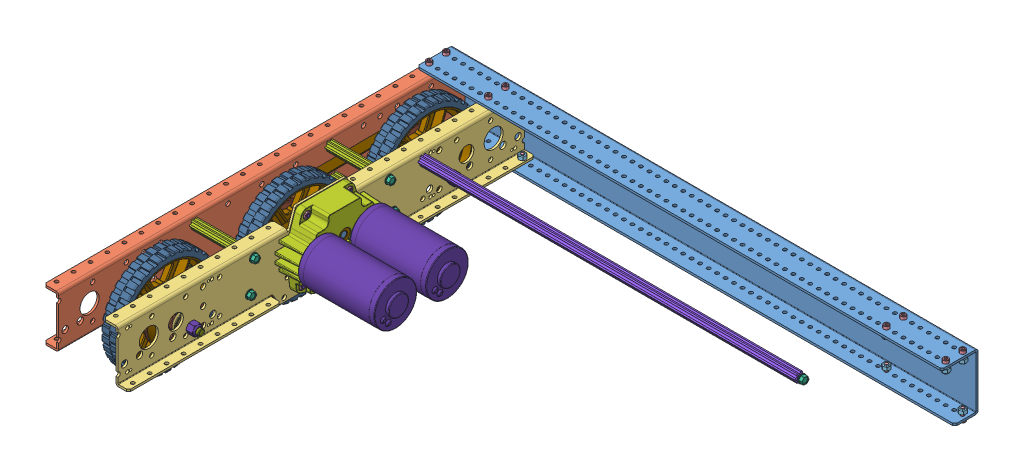
SolidWorks assembly AM14U4 Wide Half, configuration Default. Lengths in mm.
Overall size (788.5 213.52 613.54).
149 component instances, 36 part files, 33 mates.
Components (placement in the parent):
- AM14U4 Wide Frame Half-1: AM14U4 Wide Frame Half [Default] at (335.1417 50.6739 -281.2356) size (788.5 116.33 613.54)
  - am-xxxx AM14U4 End Plate-1: am-xxxx AM14U4 End Plate [Default] at (-787.4 -81.407 -3.175) x (1 0 0) z (0 -1 0) size (787.4 53.98 84.58)
  - am-xxxx AM14U4 Outside Plate Wide-1: am-xxxx AM14U4 Outside Plate Wide [DefaultSM-FLAT-PATTERN] at (-768.35 -77.216 711.962) x (0 0 -1) z (0 -1 0) size (609.6 22.23 77.72)
  - am-xxxx AM14U4 Inside Plate Wide-1: am-xxxx AM14U4 Inside Plate Wide [Default] at (-679.45 -77.216 711.962) x (0 0 -1) z (0 -1 0) size (609.6 38.1 116.33)
  - am-1002 and am-1042 10-32 x 0500 and Nylock Nut Assembly-1: am-1002 and am-1042 10-32 x 0500 and Nylock Nut Assembly [Default] at (-784.5821 -6.6363 35.2132) x (0 -1 0) z (0 0 1) size (17.53 13.8 13)
    - 10-32x0500_shcs-1: 10-32x0500_shcs [HX-SHCS 0.19-32x1.375x1-C] at (-11.4623 3.5321 3.6488) size (17.53 7.94 7.94)
    - 10-32 Nylock Nut 1-1: 10-32 Nylock Nut 1 [90631A411] at (-0.0323 3.5321 3.6488) x (0 0.381849 -0.924225) z (0 -0.924225 -0.381849) size (9.53 6.11 11)
  - am-1002 and am-1042 10-32 x 0500 and Nylock Nut Assembly-2: am-1002 and am-1042 10-32 x 0500 and Nylock Nut Assembly [Default] at (-784.5821 -6.6363 9.8132) x (0 -1 0) z (0 0 1) size (17.53 13.8 13)
    - 10-32x0500_shcs-1: 10-32x0500_shcs [HX-SHCS 0.19-32x1.375x1-C] at (-11.4623 3.5321 3.6488) size (17.53 7.94 7.94)
    - 10-32 Nylock Nut 1-1: 10-32 Nylock Nut 1 [90631A411] at (-0.0323 3.5321 3.6488) x (0 0.381849 -0.924225) z (0 -0.924225 -0.381849) size (9.53 6.11 11)
  - am-1002 and am-1042 10-32 x 0500 and Nylock Nut Assembly-3: am-1002 and am-1042 10-32 x 0500 and Nylock Nut Assembly [Default] at (-695.6821 -6.6363 35.2132) x (0 -1 0) z (0 0 1) size (17.53 13.8 13)
    - 10-32x0500_shcs-1: 10-32x0500_shcs [HX-SHCS 0.19-32x1.375x1-C] at (-11.4623 3.5321 3.6488) size (17.53 7.94 7.94)
    - 10-32 Nylock Nut 1-1: 10-32 Nylock Nut 1 [90631A411] at (-0.0323 3.5321 3.6488) x (0 0.381849 -0.924225) z (0 -0.924225 -0.381849) size (9.53 6.11 11)
  - am-1002 and am-1042 10-32 x 0500 and Nylock Nut Assembly-4: am-1002 and am-1042 10-32 x 0500 and Nylock Nut Assembly [Default] at (-695.6821 -6.6363 9.8132) x (0 -1 0) z (0 0 1) size (17.53 13.8 13)
    - 10-32x0500_shcs-1: 10-32x0500_shcs [HX-SHCS 0.19-32x1.375x1-C] at (-11.4623 3.5321 3.6488) size (17.53 7.94 7.94)
    - 10-32 Nylock Nut 1-1: 10-32 Nylock Nut 1 [90631A411] at (-0.0323 3.5321 3.6488) x (0 0.381849 -0.924225) z (0 -0.924225 -0.381849) size (9.53 6.11 11)
  - am-1002 and am-1042 10-32 x 0500 and Nylock Nut Assembly-5: am-1002 and am-1042 10-32 x 0500 and Nylock Nut Assembly [Default] at (-777.5179 -77.9457 9.8132) x (0 1 0) z (0 0 1) size (17.53 13.8 13)
    - 10-32x0500_shcs-1: 10-32x0500_shcs [HX-SHCS 0.19-32x1.375x1-C] at (-11.4623 3.5321 3.6488) size (17.53 7.94 7.94)
    - 10-32 Nylock Nut 1-1: 10-32 Nylock Nut 1 [90631A411] at (-0.0323 3.5321 3.6488) x (0 0.381849 -0.924225) z (0 -0.924225 -0.381849) size (9.53 6.11 11)
  - am-1002 and am-1042 10-32 x 0500 and Nylock Nut Assembly-6: am-1002 and am-1042 10-32 x 0500 and Nylock Nut Assembly [Default] at (-663.2179 -77.9457 9.8132) x (0 1 0) z (0 0 1) size (17.53 13.8 13)
    - 10-32x0500_shcs-1: 10-32x0500_shcs [HX-SHCS 0.19-32x1.375x1-C] at (-11.4623 3.5321 3.6488) size (17.53 7.94 7.94)
    - 10-32 Nylock Nut 1-1: 10-32 Nylock Nut 1 [90631A411] at (-0.0323 3.5321 3.6488) x (0 0.381849 -0.924225) z (0 -0.924225 -0.381849) size (9.53 6.11 11)
  - am-1002 and am-1042 10-32 x 0500 and Nylock Nut Assembly-7: am-1002 and am-1042 10-32 x 0500 and Nylock Nut Assembly [Default] at (-2.8179 -77.9457 9.8132) x (0 1 0) z (0 0 1) size (17.53 13.8 13)
    - 10-32x0500_shcs-1: 10-32x0500_shcs [HX-SHCS 0.19-32x1.375x1-C] at (-11.4623 3.5321 3.6488) size (17.53 7.94 7.94)
    - 10-32 Nylock Nut 1-1: 10-32 Nylock Nut 1 [90631A411] at (-0.0323 3.5321 3.6488) x (0 0.381849 -0.924225) z (0 -0.924225 -0.381849) size (9.53 6.11 11)
  - am-1002 and am-1042 10-32 x 0500 and Nylock Nut Assembly-8: am-1002 and am-1042 10-32 x 0500 and Nylock Nut Assembly [Default] at (-9.8821 -6.6363 9.8132) x (0 -1 0) z (0 0 1) size (17.53 13.8 13)
    - 10-32x0500_shcs-1: 10-32x0500_shcs [HX-SHCS 0.19-32x1.375x1-C] at (-11.4623 3.5321 3.6488) size (17.53 7.94 7.94)
    - 10-32 Nylock Nut 1-1: 10-32 Nylock Nut 1 [90631A411] at (-0.0323 3.5321 3.6488) x (0 0.381849 -0.924225) z (0 -0.924225 -0.381849) size (9.53 6.11 11)
  - am-1002 and am-1042 10-32 x 0500 and Nylock Nut Assembly-9: am-1002 and am-1042 10-32 x 0500 and Nylock Nut Assembly [Default] at (-9.8821 -6.6363 35.2132) x (0 -1 0) z (0 0 1) size (17.53 13.8 13)
    - 10-32x0500_shcs-1: 10-32x0500_shcs [HX-SHCS 0.19-32x1.375x1-C] at (-11.4623 3.5321 3.6488) size (17.53 7.94 7.94)
    - 10-32 Nylock Nut 1-1: 10-32 Nylock Nut 1 [90631A411] at (-0.0323 3.5321 3.6488) x (0 0.381849 -0.924225) z (0 -0.924225 -0.381849) size (9.53 6.11 11)
  - am-1002 and am-1042 10-32 x 0500 and Nylock Nut Assembly-10: am-1002 and am-1042 10-32 x 0500 and Nylock Nut Assembly [Default] at (-98.7821 -6.6363 9.8132) x (0 -1 0) z (0 0 1) size (17.53 13.8 13)
    - 10-32x0500_shcs-1: 10-32x0500_shcs [HX-SHCS 0.19-32x1.375x1-C] at (-11.4623 3.5321 3.6488) size (17.53 7.94 7.94)
    - 10-32 Nylock Nut 1-1: 10-32 Nylock Nut 1 [90631A411] at (-0.0323 3.5321 3.6488) x (0 0.381849 -0.924225) z (0 -0.924225 -0.381849) size (9.53 6.11 11)
  - am-1002 and am-1042 10-32 x 0500 and Nylock Nut Assembly-11: am-1002 and am-1042 10-32 x 0500 and Nylock Nut Assembly [Default] at (-98.7821 -6.6363 35.2132) x (0 -1 0) z (0 0 1) size (17.53 13.8 13)
    - 10-32x0500_shcs-1: 10-32x0500_shcs [HX-SHCS 0.19-32x1.375x1-C] at (-11.4623 3.5321 3.6488) size (17.53 7.94 7.94)
    - 10-32 Nylock Nut 1-1: 10-32 Nylock Nut 1 [90631A411] at (-0.0323 3.5321 3.6488) x (0 0.381849 -0.924225) z (0 -0.924225 -0.381849) size (9.53 6.11 11)
  - am-1002 and am-1042 10-32 x 0500 and Nylock Nut Assembly-12: am-1002 and am-1042 10-32 x 0500 and Nylock Nut Assembly [Default] at (-117.1179 -77.9457 9.8132) x (0 1 0) z (0 0 1) size (17.53 13.8 13)
    - 10-32x0500_shcs-1: 10-32x0500_shcs [HX-SHCS 0.19-32x1.375x1-C] at (-11.4623 3.5321 3.6488) size (17.53 7.94 7.94)
    - 10-32 Nylock Nut 1-1: 10-32 Nylock Nut 1 [90631A411] at (-0.0323 3.5321 3.6488) x (0 0.381849 -0.924225) z (0 -0.924225 -0.381849) size (9.53 6.11 11)
  - FHTS 0.25-20-0.75-1: FHTS 0.25-20-0.75 [FHTS 0.25-20-G-0.75-C] at (-768.35 -59.6687 198.0365) size (24.64 12.19 12.19)
  - FHTS 0.25-20-0.75-2: FHTS 0.25-20-0.75 [FHTS 0.25-20-G-0.75-C] at (-768.35 -14.986 203.962) size (24.64 12.19 12.19)
  - FHTS 0.25-20-0.75-3: FHTS 0.25-20-0.75 [FHTS 0.25-20-G-0.75-C] at (-768.35 -14.986 407.162) size (24.64 12.19 12.19)
  - FHTS 0.25-20-0.75-4: FHTS 0.25-20-0.75 [FHTS 0.25-20-G-0.75-C] at (-768.35 -59.6687 413.0875) size (24.64 12.19 12.19)
  - FHTS 0.25-20-0.75-5: FHTS 0.25-20-0.75 [FHTS 0.25-20-G-0.75-C] at (-676.275 -59.6687 413.0875) x (-1 0 0) z (0 0.924225 0.381849) size (24.64 12.19 12.19)
  - FHTS 0.25-20-0.75-6: FHTS 0.25-20-0.75 [FHTS 0.25-20-G-0.75-C] at (-676.275 -14.986 407.162) x (-1 0 0) z (0 0.924225 0.381849) size (24.64 12.19 12.19)
  - FHTS 0.25-20-0.75-7: FHTS 0.25-20-0.75 [FHTS 0.25-20-G-0.75-C] at (-676.275 -14.986 203.962) x (-1 0 0) z (0 0.924225 0.381849) size (24.64 12.19 12.19)
  - FHTS 0.25-20-0.75-8: FHTS 0.25-20-0.75 [FHTS 0.25-20-G-0.75-C] at (-676.275 -59.6687 198.0365) x (-1 0 0) z (0 0.924225 0.381849) size (24.64 12.19 12.19)
  - 3.375in Churro-1: 3.375in Churro [Default] at (-679.45 -59.6687 198.0365) x (0 0 1) z (-1 0 0) size (14.66 12.7 85.72)
  - 3.375in Churro-2: 3.375in Churro [Default] at (-679.45 -14.986 203.962) x (0 0 1) z (-1 0 0) size (14.66 12.7 85.72)
  - 3.375in Churro-3: 3.375in Churro [Default] at (-679.45 -14.986 407.162) x (0 0 1) z (-1 0 0) size (14.66 12.7 85.72)
  - 3.375in Churro-4: 3.375in Churro [Default] at (-679.45 -59.6687 413.0875) x (0 0 1) z (-1 0 0) size (14.66 12.7 85.72)
  - 22.25in Churro-1: 22.25in Churro [Default] at (-393.7 -14.986 153.162) x (0 0 -1) z (1 0 0) size (14.66 12.7 565.15)
  - FHTS 0.25-20-0.75-9: FHTS 0.25-20-0.75 [FHTS 0.25-20-G-0.75-C] at (-107.95 -14.986 153.162) x (-1 0 0) z (0 0.924225 0.381849) size (24.64 12.19 12.19)
- 6 HiGrip with bearings, pulleys and spacers-1: 6 HiGrip with bearings, pulleys and spacers [Default] at (-418.7948 -84.3541 86.993) size (85.56 152.4 152.4)
  - 6 HiGrip Asm Rev II-1: 6 HiGrip Asm Rev II [Default] at (83.7987 67.439 110.9939) size (35.05 152.4 152.4)
    - 6 wheel Rev 4-1: 6 wheel Rev 4 [Default] at (-52.6446 9.4231 21.378) size (35.05 132.08 132.08)
    - 6 wheel tread II-1: 6 wheel tread II [Default] at (-65.3446 9.4231 21.378) x (0 0 -1) z (1 0 0) size (152.4 152.4 25.58)
  - 42 tooth HTD Pulley half 2014-1: 42 tooth HTD Pulley half 2014 [Default] at (47.6006 76.862 132.3719) x (1 0 0) z (0 -0.5 0.866025) size (13 74.23 74.23)
  - 42 tooth HTD Pulley half 2014-2: 42 tooth HTD Pulley half 2014 [Default] at (64.263 76.862 132.3719) x (-1 0 0) z (0 -0.499927 0.866067) size (13 74.23 74.23)
  - 1614Z Bearing-1: 1614Z Bearing [Default] at (62.612 76.862 132.3719) x (0 -0.157148 -0.987575) z (-1 0 0) size (28.57 28.57 9.53)
  - 10-24 Hex Washer Rolling x 1.25-1: 10-24 Hex Washer Rolling x 1.25 [93882A213] at (63.247 76.8605 108.5602) x (0 0 -1) z (1 0 0) size (10.52 10.52 35.59)
  - 10-24 Hex Washer Rolling x 1.25-2: 10-24 Hex Washer Rolling x 1.25 [93882A213] at (63.247 97.4833 120.4656) x (0 0 -1) z (1 0 0) size (10.52 10.52 35.59)
  - 10-24 Hex Washer Rolling x 1.25-3: 10-24 Hex Washer Rolling x 1.25 [93882A213] at (63.247 56.2398 144.2799) x (0 0 -1) z (1 0 0) size (10.52 10.52 35.59)
  - 10-24 Hex Washer Rolling x 1.25-4: 10-24 Hex Washer Rolling x 1.25 [93882A213] at (63.247 76.8625 156.1852) x (0 -0.95788 -0.287168) z (1 0 0) size (10.52 10.52 35.59)
  - 10-24 Hex Washer Rolling x 1.25-5: 10-24 Hex Washer Rolling x 1.25 [93882A213] at (63.247 97.4843 144.2781) x (0 -0.868976 0.494854) z (1 0 0) size (10.52 10.52 35.59)
  - 10-24 Hex Washer Rolling x 1.25-6: 10-24 Hex Washer Rolling x 1.25 [93882A213] at (63.247 56.2388 120.4674) x (0 -0.977348 -0.211637) z (1 0 0) size (10.52 10.52 35.59)
  - am-1306 spacer 0280 WashersUSA 13RS052001-1: am-1306 spacer 0280 WashersUSA 13RS052001 [Default] at (74.4865 76.862 132.3719) x (0 -0.35357 0.935408) z (-1 0 0) size (13.16 13.16 7.11)
  - 1614Z Bearing-2: 1614Z Bearing [Default] at (15.2791 76.862 132.3719) x (0 0.155433 -0.987846) z (-1 0 0) size (28.57 28.57 9.53)
  - am-1307 850 long 380 id-1: am-1307 850 long 380 id [Default] at (10.5166 76.862 132.3719) x (0 0.971418 -0.237374) z (0 0.237374 0.971418) size (19.05 21.59 19.05)
- 6 HiGrip with bearings, pulleys and spacers-2: 6 HiGrip with bearings, pulleys and spacers [Default] at (-355.3817 51.5414 -29.4849) x (-1 0 0) z (0 -0.796812 -0.604227) size (85.56 152.4 152.4)
  - 6 HiGrip Asm Rev II-1: 6 HiGrip Asm Rev II [Default] at (83.7987 67.439 110.9939) size (35.05 152.4 152.4)
    - 6 wheel Rev 4-1: 6 wheel Rev 4 [Default] at (-52.6446 9.4231 21.378) size (35.05 132.08 132.08)
    - 6 wheel tread II-1: 6 wheel tread II [Default] at (-65.3446 9.4231 21.378) x (0 0 -1) z (1 0 0) size (152.4 152.4 25.58)
  - 42 tooth HTD Pulley half 2014-1: 42 tooth HTD Pulley half 2014 [Default] at (47.6006 76.862 132.3719) x (1 0 0) z (0 -0.5 0.866025) size (13 74.23 74.23)
  - 42 tooth HTD Pulley half 2014-2: 42 tooth HTD Pulley half 2014 [Default] at (64.263 76.862 132.3719) x (-1 0 0) z (0 -0.499927 0.866067) size (13 74.23 74.23)
  - 1614Z Bearing-1: 1614Z Bearing [Default] at (62.612 76.862 132.3719) x (0 -0.157148 -0.987575) z (-1 0 0) size (28.57 28.57 9.53)
  - 10-24 Hex Washer Rolling x 1.25-1: 10-24 Hex Washer Rolling x 1.25 [93882A213] at (63.247 76.8605 108.5602) x (0 0 -1) z (1 0 0) size (10.52 10.52 35.59)
  - 10-24 Hex Washer Rolling x 1.25-2: 10-24 Hex Washer Rolling x 1.25 [93882A213] at (63.247 97.4833 120.4656) x (0 0 -1) z (1 0 0) size (10.52 10.52 35.59)
  - 10-24 Hex Washer Rolling x 1.25-3: 10-24 Hex Washer Rolling x 1.25 [93882A213] at (63.247 56.2398 144.2799) x (0 0 -1) z (1 0 0) size (10.52 10.52 35.59)
  - 10-24 Hex Washer Rolling x 1.25-4: 10-24 Hex Washer Rolling x 1.25 [93882A213] at (63.247 76.8625 156.1852) x (0 -0.95788 -0.287168) z (1 0 0) size (10.52 10.52 35.59)
  - 10-24 Hex Washer Rolling x 1.25-5: 10-24 Hex Washer Rolling x 1.25 [93882A213] at (63.247 97.4843 144.2781) x (0 -0.868976 0.494854) z (1 0 0) size (10.52 10.52 35.59)
  - 10-24 Hex Washer Rolling x 1.25-6: 10-24 Hex Washer Rolling x 1.25 [93882A213] at (63.247 56.2388 120.4674) x (0 -0.977348 -0.211637) z (1 0 0) size (10.52 10.52 35.59)
  - am-1306 spacer 0280 WashersUSA 13RS052001-1: am-1306 spacer 0280 WashersUSA 13RS052001 [Default] at (74.4865 76.862 132.3719) x (0 -0.35357 0.935408) z (-1 0 0) size (13.16 13.16 7.11)
  - 1614Z Bearing-2: 1614Z Bearing [Default] at (15.2791 76.862 132.3719) x (0 0.155433 -0.987846) z (-1 0 0) size (28.57 28.57 9.53)
  - am-1307 850 long 380 id-1: am-1307 850 long 380 id [Default] at (10.5166 76.862 132.3719) x (0 0.971418 -0.237374) z (0 0.237374 0.971418) size (19.05 21.59 19.05)
- 375-16 x 4.25 Hex Bolt-1: 375-16 x 4.25 Hex Bolt [HFBOLT 0.375-16x2.5x1-C] at (-439.3805 -7.4921 -170.7121) size (114.12 16.48 14.27)
- 375-16 x 4.25 Hex Bolt-2: 375-16 x 4.25 Hex Bolt [HFBOLT 0.375-16x2.5x1-C] at (-439.3805 -7.4921 219.3649) size (114.12 16.48 14.27)
- 3-8-16 NyLock Nut - Mcm 95615A140-1: 3-8-16 NyLock Nut - Mcm 95615A140 [95615A140] at (-341.1333 -7.4921 -170.7121) x (0 -1 0) z (0 0 1) size (14.29 12 16.5)
- 3-8-16 NyLock Nut - Mcm 95615A140-2: 3-8-16 NyLock Nut - Mcm 95615A140 [95615A140] at (-341.1333 -7.4921 219.3649) x (0 -1 0) z (0 0 1) size (14.29 12 16.5)
- FR8ZZ Hex Bearing-1: FR8ZZ Hex Bearing [Default] at (-436.4366 -9.2701 24.3264) x (0 0 -1) z (1 0 0) size (31.12 31.12 7.93)
- am-2598_107 2016 KOP Toughbox Mini-1: am-2598_107 2016 KOP Toughbox Mini [Default] at (-391.675 -19.3401 115.4272) x (0 0.001296 0.999999) z (-1 0 0) size (140.05 121.81 142.29)
  - Toughbox d07-1: Toughbox d07 [Default] at (-88.5589 93.4503 -52.3959) x (-0.336928 0.94153 0) z (0.94153 0.336928 0) size (11 38.23 9.52)
  - Toughbox d05-1: Toughbox d05 [Default] at (-91.0349 50.9043 -67.5597) x (-0.336928 0.94153 0) z (0 0 -1) size (65.97 66.04 10.16)
  - FR6ZZ Bearing-1: FR6ZZ Bearing [Default] at (-96.247 60.278 -52.5991) x (-0.893862 0.448342 0) z (0 0 1) size (24.69 24.69 7.16)
  - 10-32 Nylock Nut-1: 10-32 Nylock Nut [Default] at (-129.8464 -8.0737 -56.3837) x (0.501678 0.865055 0) z (0 0 -1) size (10.18 11.01 7.1)
  - 10-32 Nylock Nut-2: 10-32 Nylock Nut [Default] at (-59.2462 80.7349 -56.3837) x (0.999999 -0.001296 0) z (0 0 -1) size (10.18 11.01 7.1)
  - 10-32 Nylock Nut-3: 10-32 Nylock Nut [Default] at (-122.7461 80.8172 -56.3837) x (0.500567 0.865698 0) z (0 0 -1) size (10.18 11.01 7.1)
  - 10-32 Nylock Nut-4: 10-32 Nylock Nut [Default] at (-52.3764 -8.1741 -56.3837) x (-0.501678 -0.865055 0) z (0 0 -1) size (10.18 11.01 7.1)
  - 5-16 washer-1: 5-16 washer [Default] at (-52.3162 38.3079 -77.7705) x (0.38418 -0.923258 0) z (0 0 -1) size (17.53 17.53 1.47)
  - 5-16 washer-2: 5-16 washer [Default] at (-52.3162 38.3079 -76.2973) x (0.897267 -0.441488 0) z (0 0 -1) size (17.53 17.53 1.47)
  - 5-16 washer-3: 5-16 washer [Default] at (-129.7861 38.4083 -77.7705) x (-0.990116 0.140253 0) z (0 0 1) size (17.53 17.53 1.47)
  - 5-16 washer-4: 5-16 washer [Default] at (-129.7861 38.4083 -79.2437) x (-0.681761 0.731575 0) z (0 0 1) size (17.53 17.53 1.47)
  - Toughbox d09-1: Toughbox d09 [Default] at (-52.3162 38.3079 -63.5973) x (0.910249 -0.414061 0) z (0 0 -1) size (20.03 20.32 12.7)
  - Toughbox d09-2: Toughbox d09 [Default] at (-129.7861 38.4083 -63.5973) x (0.075368 -0.997156 0) z (0 0 -1) size (20.03 20.32 12.7)
  - TM Housing-1: TM Housing [Default] at (-91.0876 10.1882 -86.3557) x (0.999999 -0.001296 0) z (0 0 1) size (139.9 118.55 41.54)
  - SHCS 10-32 x 0.625-1: SHCS 10-32 x 0.625 [Default] at (-52.2832 63.7078 -74.4685) x (-0.564778 -0.825243 0) z (-0.825243 0.564778 0) size (7.82 20.65 7.82)
  - SHCS 10-32 x 0.625-2: SHCS 10-32 x 0.625 [Default] at (-122.7461 80.8172 -42.5915) x (0.507484 -0.861661 0) z (-0.861661 -0.507484 0) size (7.82 20.65 7.82)
  - SHCS 10-32 x 0.625-3: SHCS 10-32 x 0.625 [Default] at (-52.3764 -8.1741 -42.5915) x (0.507484 -0.861661 0) z (-0.861661 -0.507484 0) size (7.82 20.65 7.82)
  - SHCS 10-32 x 0.625-4: SHCS 10-32 x 0.625 [Default] at (-129.8464 -8.0737 -42.5915) x (0.507484 -0.861661 0) z (-0.861661 -0.507484 0) size (7.82 20.65 7.82)
  - SHCS 10-32 x 0.625-5: SHCS 10-32 x 0.625 [Default] at (-59.2462 80.7349 -42.5915) x (0.740711 -0.671824 0) z (-0.671824 -0.740711 0) size (7.82 20.65 7.82)
  - SHCS 10-32 x 0.625-6: SHCS 10-32 x 0.625 [Default] at (-52.3491 12.9079 -74.4685) x (-0.564778 -0.825243 0) z (-0.825243 0.564778 0) size (7.82 20.65 7.82)
  - SHCS 10-32 x 0.625-7: SHCS 10-32 x 0.625 [Default] at (-129.7532 63.8083 -74.4685) x (-0.966277 -0.257503 0) z (-0.257503 0.966277 0) size (7.82 20.65 7.82)
  - SHCS 10-32 x 0.625-8: SHCS 10-32 x 0.625 [Default] at (-129.819 13.0083 -74.4685) x (-0.99652 0.083357 0) z (0.083357 0.99652 0) size (7.82 20.65 7.82)
  - R6ZZ Bearing-3: R6ZZ Bearing [Default] at (-91.0349 50.9043 -84.8317) x (0.958138 -0.286306 0) z (0 0 1) size (22.23 22.23 7.11)
  - R6ZZ Bearing-4: R6ZZ Bearing [Default] at (-91.0876 10.1882 -84.8317) x (-0.328282 -0.94458 0) z (0 0 1) size (22.23 22.23 7.11)
  - 8mm spring clip-1: 8mm spring clip [Default] at (-129.7861 38.4083 -63.5973) x (0 0 1) z (-1 0 0) size (1.09 14.83 14.83)
  - 8mm spring clip-2: 8mm spring clip [Default] at (-52.3162 38.3079 -63.5973) x (0 0 1) z (-1 0 0) size (1.09 14.83 14.83)
  - 500 E-klip-1: 500 E-klip [Default] at (-91.0876 10.1882 -64.4355) x (0.996411 -0.084651 0) z (0 0 1) size (19.07 20.96 1.27)
  - FR8ZZ Hex Bearing-1: FR8ZZ Hex Bearing [Default] at (-91.0876 10.1882 -44.6717) x (-0.5 0.866025 0) z (0 0 -1) size (31.12 31.12 7.93)
  - 16t 20dp 375h with teeth-1: 16t 20dp 375h with teeth [Default] at (-91.0349 50.9043 -67.5597) x (0 0 1) z (-0.983853 0.178977 0) size (15.19 22.57 22.57)
  - 48t 20dp 500h with teeth-1: 48t 20dp 500h with teeth [Default] at (-91.0876 10.1882 -63.1655) x (0 0 1) z (-1 0 0) size (10.21 63.42 63.42)
  - TB Output Shaft Hex L-Base 2-1: TB Output Shaft Hex L-Base 2 [Default] at (-52.7805 -6.4809 -52.3197) x (1 0 0) z (0 -1 0) size (14.66 142.29 12.7)
- 6 HiGrip with hub and double pulley-1: 6 HiGrip with hub and double pulley [Default] at (-355.308 143.7987 24.5073) x (-1 0 0) z (0 -0.865376 0.501122) size (81.42 152.4 152.4)
  - 6 HiGrip Asm Rev II-1: 6 HiGrip Asm Rev II [Default] at (83.7987 67.439 110.9939) size (35.05 152.4 152.4)
    - 6 wheel Rev 4-1: 6 wheel Rev 4 [Default] at (-52.6446 9.4231 21.378) size (35.05 132.08 132.08)
    - 6 wheel tread II-1: 6 wheel tread II [Default] at (-65.3446 9.4231 21.378) x (0 0 -1) z (1 0 0) size (152.4 152.4 25.58)
  - 42 tooth HTD Pulley half 2014-1: 42 tooth HTD Pulley half 2014 [Default] at (47.6006 76.862 132.3719) x (1 0 0) z (0 -0.5 0.866025) size (13 74.23 74.23)
  - 42 tooth HTD Pulley half 2014-2: 42 tooth HTD Pulley half 2014 [Default] at (64.263 76.862 132.3719) x (-1 0 0) z (0 -0.499927 0.866067) size (13 74.23 74.23)
  - 10-24 Hex Washer Rolling x 1.25-1: 10-24 Hex Washer Rolling x 1.25 [93882A213] at (63.247 76.8605 108.5602) x (0 0 -1) z (1 0 0) size (10.52 10.52 35.59)
  - 10-24 Hex Washer Rolling x 1.25-2: 10-24 Hex Washer Rolling x 1.25 [93882A213] at (63.247 97.4833 120.4656) x (0 0 -1) z (1 0 0) size (10.52 10.52 35.59)
  - 10-24 Hex Washer Rolling x 1.25-3: 10-24 Hex Washer Rolling x 1.25 [93882A213] at (63.247 56.2398 144.2799) x (0 0 -1) z (1 0 0) size (10.52 10.52 35.59)
  - 10-24 Hex Washer Rolling x 1.25-4: 10-24 Hex Washer Rolling x 1.25 [93882A213] at (63.247 76.8625 156.1852) x (0 -0.95788 -0.287168) z (1 0 0) size (10.52 10.52 35.59)
  - 10-24 Hex Washer Rolling x 1.25-5: 10-24 Hex Washer Rolling x 1.25 [93882A213] at (63.247 97.4843 144.2781) x (0 -0.868976 0.494854) z (1 0 0) size (10.52 10.52 35.59)
  - 10-24 Hex Washer Rolling x 1.25-6: 10-24 Hex Washer Rolling x 1.25 [93882A213] at (63.247 56.2388 120.4674) x (0 -0.748729 -0.662876) z (1 0 0) size (10.52 10.52 35.59)
  - 42 tooth HTD Pulley half 2014-3: 42 tooth HTD Pulley half 2014 [Default] at (-1.9548 76.8628 132.3714) x (1 0 0) z (0 -1 -0.000063) size (13 74.23 74.23)
  - 42 tooth HTD Pulley half 2014-4: 42 tooth HTD Pulley half 2014 [Default] at (14.7076 76.8628 132.3714) x (-1 0 0) z (0 -1 0.000021) size (13 74.23 74.23)
  - 500EX Hex Hub-1: 500EX Hex Hub [Default] at (-8.3048 76.8628 132.3714) x (0 -0.866025 -0.5) z (0 -0.5 0.866025) size (55.37 25.4 51.33)
  - 10-24 Hex Washer Rolling x 1.25-7: 10-24 Hex Washer Rolling x 1.25 [93882A213] at (-5.2568 97.485 120.4652) x (0 0 1) z (-1 0 0) size (10.52 10.52 35.59)
  - 10-24 Hex Washer Rolling x 1.25-8: 10-24 Hex Washer Rolling x 1.25 [93882A213] at (-5.2568 76.8628 108.5589) x (0 0 1) z (-1 0 0) size (10.52 10.52 35.59)
  - 10-24 Hex Washer Rolling x 1.25-9: 10-24 Hex Washer Rolling x 1.25 [93882A213] at (-5.2568 56.2406 120.4652) x (0 0 1) z (-1 0 0) size (10.52 10.52 35.59)
  - 10-24 Hex Washer Rolling x 1.25-10: 10-24 Hex Washer Rolling x 1.25 [93882A213] at (-5.2568 97.485 144.2777) x (0 -0.99374 -0.111715) z (-1 0 0) size (10.52 10.52 35.59)
  - 10-24 Hex Washer Rolling x 1.25-11: 10-24 Hex Washer Rolling x 1.25 [93882A213] at (-5.2568 56.2406 144.2777) x (0 -0.138911 0.990305) z (-1 0 0) size (10.52 10.52 35.59)
  - 10-24 Hex Washer Rolling x 1.25-12: 10-24 Hex Washer Rolling x 1.25 [93882A213] at (-5.2568 76.8628 156.1839) x (0 -0.98811 -0.15375) z (-1 0 0) size (10.52 10.52 35.59)
  - am-1305 500 Hex Spacer-1: am-1305 500 Hex Spacer [Default] at (57.8495 76.862 132.3719) x (0 -0.866025 -0.5) z (0 -0.5 0.866025) size (28.55 14.48 28.55)
- CIM Motor SW-1: CIM Motor SW [Default] at (-286.2693 54.4599 -123.7048) x (0 -1 0) z (-1 0 0) size (64.01 64.01 154.93)
- CIM Motor SW-2: CIM Motor SW [Default] at (-286.2693 54.4599 -46.2348) x (0 -1 0) z (-1 0 0) size (64.01 64.01 154.93)
- 600-5M-15 v2-1: 600-5M-15 v2 [Default] at (-370.0156 -7.4921 219.3649) x (0 -0.009116 -0.999958) z (0 -0.999958 0.009116) size (268.12 15 73.08)
- 600-5M-15 v2-2: 600-5M-15 v2 [Default] at (-402.9086 -7.4921 -170.7121) x (0 -0.009116 0.999958) z (0 -0.999958 -0.009116) size (268.12 15 73.08)
Mates (geometry in assembly coordinates):
- Coincident1: coincident: plane of AM14U4 Wide Frame Half-1/am-xxxx AM14U4 Inside Plate Wide-1 through (-344.3083 43.3079 430.7264) normal (-1 0 0); plane of 6 HiGrip with bearings, pulleys and spacers-1/am-1306 spacer 0280 WashersUSA 13RS052001-1 through (-344.3083 -7.4921 219.3649) normal (1 0 0)
- Concentric1: concentric: cylinder of AM14U4 Wide Frame Half-1/am-xxxx AM14U4 Inside Plate Wide-1 through (-363.3583 -7.4921 219.3649) axis (1 0 0) radius 4.826; cylinder of 6 HiGrip with bearings, pulleys and spacers-1/am-1306 spacer 0280 WashersUSA 13RS052001-1 through (-351.4203 -7.4921 219.3649) axis (1 0 0) radius 4.8514
- Coincident2: coincident: plane of AM14U4 Wide Frame Half-1/am-xxxx AM14U4 Inside Plate Wide-1 through (-344.3083 43.3079 430.7264) normal (-1 0 0); plane of 6 HiGrip with bearings, pulleys and spacers-2/am-1307 850 long 380 id-1 through (-344.3083 -7.4921 -170.7121) normal (1 0 0)
- Concentric2: concentric: cylinder of AM14U4 Wide Frame Half-1/am-xxxx AM14U4 Inside Plate Wide-1 through (-363.3583 -7.4921 -170.7121) axis (1 0 0) radius 4.826; cylinder of 6 HiGrip with bearings, pulleys and spacers-2/am-1307 850 long 380 id-1 through (-344.3083 -7.4921 -170.7121) axis (-1 0 0) radius 4.826
- Concentric31: concentric: cylinder of AM14U4 Wide Frame Half-1/am-xxxx AM14U4 Outside Plate Wide-1 through (-541.1593 -7.4921 -170.7121) axis (1 0 0) radius 4.826; cylinder of 375-16 x 4.25 Hex Bolt-1 through (-439.3805 -7.4921 -170.7121) axis (-1 0 0) radius 7.1374
- Coincident31: coincident: plane of AM14U4 Wide Frame Half-1/am-xxxx AM14U4 Outside Plate Wide-1 through (-433.2083 43.3079 430.7264) normal (-1 0 0); plane of 375-16 x 4.25 Hex Bolt-1 through (-433.2083 0.7495 -170.7121) normal (1 0 0)
- Concentric41: concentric: cylinder of AM14U4 Wide Frame Half-1/am-xxxx AM14U4 Outside Plate Wide-1 through (-541.1593 -7.4921 219.3649) axis (1 0 0) radius 4.826; cylinder of 375-16 x 4.25 Hex Bolt-2 through (-439.3805 -7.4921 219.3649) axis (-1 0 0) radius 7.1374
- Coincident41: coincident: plane of AM14U4 Wide Frame Half-1/am-xxxx AM14U4 Outside Plate Wide-1 through (-433.2083 43.3079 430.7264) normal (-1 0 0); plane of 375-16 x 4.25 Hex Bolt-2 through (-433.2083 0.7495 219.3649) normal (1 0 0)
- Coincident5: coincident: plane of AM14U4 Wide Frame Half-1/am-xxxx AM14U4 Inside Plate Wide-1 through (-341.1333 43.3079 430.7264) normal (1 0 0); plane of 3-8-16 NyLock Nut - Mcm 95615A140-1 through (-341.1333 -0.3483 -183.0855) normal (-1 0 0)
- Coincident6: coincident: plane of AM14U4 Wide Frame Half-1/am-xxxx AM14U4 Inside Plate Wide-1 through (-341.1333 43.3079 430.7264) normal (1 0 0); plane of 3-8-16 NyLock Nut - Mcm 95615A140-2 through (-341.1333 -0.3483 206.9915) normal (-1 0 0)
- Concentric5: concentric: cylinder of 375-16 x 4.25 Hex Bolt-2 through (-439.3805 -7.4921 219.3649) axis (-1 0 0) radius 4.7625; cylinder of 3-8-16 NyLock Nut - Mcm 95615A140-2 through (-331.466 -7.4921 219.3649) axis (-1 0 0) radius 4.0291
- Concentric6: concentric: cylinder of 375-16 x 4.25 Hex Bolt-1 through (-439.3805 -7.4921 -170.7121) axis (-1 0 0) radius 4.7625; cylinder of 3-8-16 NyLock Nut - Mcm 95615A140-1 through (-331.466 -7.4921 -170.7121) axis (-1 0 0) radius 4.0291
- Concentric71: concentric: cylinder of AM14U4 Wide Frame Half-1/am-xxxx AM14U4 Outside Plate Wide-1 through (-433.2083 -9.2701 24.3264) axis (1 0 0) radius 14.2875; cylinder of FR8ZZ Hex Bearing-1 through (-428.5093 -9.2701 24.3264) axis (-1 0 0) radius 13.97
- Coincident71: coincident: plane of AM14U4 Wide Frame Half-1/am-xxxx AM14U4 Outside Plate Wide-1 through (-430.0333 43.3079 430.7264) normal (1 0 0); plane of FR8ZZ Hex Bearing-1 through (-430.0333 -9.2701 10.3564) normal (-1 0 0)
- Parallel1: parallel: plane of AM14U4 Wide Frame Half-1/am-xxxx AM14U4 Outside Plate Wide-1 through (-433.2083 47.2449 -382.0736) normal (0 1 0); plane of FR8ZZ Hex Bearing-1 through (-428.5093 -15.6201 20.6602) normal (0 1 0)
- Concentric8: concentric: cylinder of AM14U4 Wide Frame Half-1/am-xxxx AM14U4 Inside Plate Wide-1 through (-344.3083 -9.2701 24.3264) axis (1 0 0) radius 14.2875; cylinder of am-2598_107 2016 KOP Toughbox Mini-1/FR8ZZ Hex Bearing-1 through (-339.0759 -9.2701 24.3264) axis (-1 0 0) radius 14.2875
- Parallel2: parallel: plane of AM14U4 Wide Frame Half-1/am-xxxx AM14U4 Inside Plate Wide-1 through (-341.1333 70.7399 -23.2986) normal (0 1 0); line of am-2598_107 2016 KOP Toughbox Mini-1/TM Housing-1 through (-340.6076 70.2972 -7.4236) axis (0 0 1)
- Coincident10: coincident: plane of AM14U4 Wide Frame Half-1/am-xxxx AM14U4 Inside Plate Wide-1 through (-341.1333 43.3079 430.7264) normal (1 0 0); plane of am-2598_107 2016 KOP Toughbox Mini-1/TM Housing-1 through (-341.1333 -9.2701 24.3264) normal (-1 0 0)
- Concentric9: concentric: cylinder of am-2598_107 2016 KOP Toughbox Mini-1/FR8ZZ Hex Bearing-1 through (-339.0759 -9.2701 24.3264) axis (-1 0 0) radius 14.2875; cylinder of 6 HiGrip with hub and double pulley-1/500EX Hex Hub-1 through (-320.8736 -9.2701 24.3264) axis (-1 0 0) radius 9.2382
- Parallel3: parallel: plane of am-2598_107 2016 KOP Toughbox Mini-1/TB Output Shaft Hex L-Base 2-1 through (-313.9553 -2.9153 27.9843) normal (0 0.999999 -0.001296); plane of 6 HiGrip with hub and double pulley-1/500EX Hex Hub-1 through (-347.0032 -15.6375 20.6611) normal (0 0.999999 -0.001296)
- Coincident12: coincident: plane of am-2598_107 2016 KOP Toughbox Mini-1/FR8ZZ Hex Bearing-1 through (-347.0032 -9.2701 24.3264) normal (-1 0 0); plane of 6 HiGrip with hub and double pulley-1/500EX Hex Hub-1 through (-347.0032 -9.2701 24.3264) normal (1 0 0)
- Coincident13: coincident: plane of CIM Motor SW-1 through (-305.3193 18.8999 -14.4086) normal (-1 0 0); plane of CIM Motor SW-2 through (-305.3193 18.8999 63.0614) normal (-1 0 0)
- Concentric10: concentric: cylinder of am-2598_107 2016 KOP Toughbox Mini-1/TM Housing-1 through (-341.1333 18.8999 -14.4086) axis (-1 0 0) radius 10.414; cylinder of CIM Motor SW-1 through (-297.0897 18.8999 -14.4086) axis (1 0 0) radius 32.004
- Concentric11: concentric: cylinder of am-2598_107 2016 KOP Toughbox Mini-1/TM Housing-1 through (-341.1333 18.8999 63.0614) axis (-1 0 0) radius 10.414; cylinder of CIM Motor SW-2 through (-297.0897 18.8999 63.0614) axis (1 0 0) radius 32.004
- Concentric12: concentric: cylinder of am-2598_107 2016 KOP Toughbox Mini-1/SHCS 10-32 x 0.625-6 through (-296.5563 -6.5001 63.0614) axis (-1 0 0) radius 2.3876; cylinder of CIM Motor SW-2 through (-305.3193 -6.5001 63.0614) axis (-1 0 0) radius 2.0193
- Concentric13: concentric: cylinder of am-2598_107 2016 KOP Toughbox Mini-1/SHCS 10-32 x 0.625-8 through (-296.5563 -6.5001 -14.4086) axis (-1 0 0) radius 2.3876; circle of CIM Motor SW-1
- Coincident14: coincident: plane of am-2598_107 2016 KOP Toughbox Mini-1/TM Housing-1 through (-305.3193 -9.2701 24.3264) normal (1 0 0); plane of CIM Motor SW-2 through (-305.3193 18.8999 63.0614) normal (-1 0 0)
- Concentric14: concentric: cylinder of 6 HiGrip with bearings, pulleys and spacers-1/am-1307 850 long 380 id-1 through (-429.8682 -7.4921 219.3649) axis (1 0 0) radius 9.525; cylinder of 600-5M-15 v2-1 through (-355.0156 -7.4921 219.3649) axis (-1 0 0) radius 35.0139
- Concentric15: concentric: cylinder of FR8ZZ Hex Bearing-1 through (-428.5093 -9.2701 24.3264) axis (-1 0 0) radius 14.2875; cylinder of 600-5M-15 v2-1 through (-355.0156 -9.2701 24.3264) axis (-1 0 0) radius 35.0139
- Coincident15: coincident: plane of 6 HiGrip with hub and double pulley-1/42 tooth HTD Pulley half 2014-4 through (-370.0156 -9.2701 24.3264) normal (1 0 0); plane of 600-5M-15 v2-1 through (-370.0156 -7.4921 219.3649) normal (-1 0 0)
- Concentric16: concentric: cylinder of 6 HiGrip with bearings, pulleys and spacers-2/am-1307 850 long 380 id-1 through (-344.3083 -7.4921 -170.7121) axis (-1 0 0) radius 9.525; cylinder of 600-5M-15 v2-2 through (-417.9086 -7.4921 -170.7121) axis (1 0 0) radius 35.0139
- Concentric17: concentric: cylinder of FR8ZZ Hex Bearing-1 through (-428.5093 -9.2701 24.3264) axis (-1 0 0) radius 14.2875; cylinder of 600-5M-15 v2-2 through (-417.9086 -9.2701 24.3264) axis (1 0 0) radius 35.0139
- Coincident16: coincident: plane of 6 HiGrip with hub and double pulley-1/42 tooth HTD Pulley half 2014-1 through (-402.9086 -9.2701 24.3272) normal (-1 0 0); plane of 600-5M-15 v2-2 through (-402.9086 -7.4921 -170.7121) normal (1 0 0)
